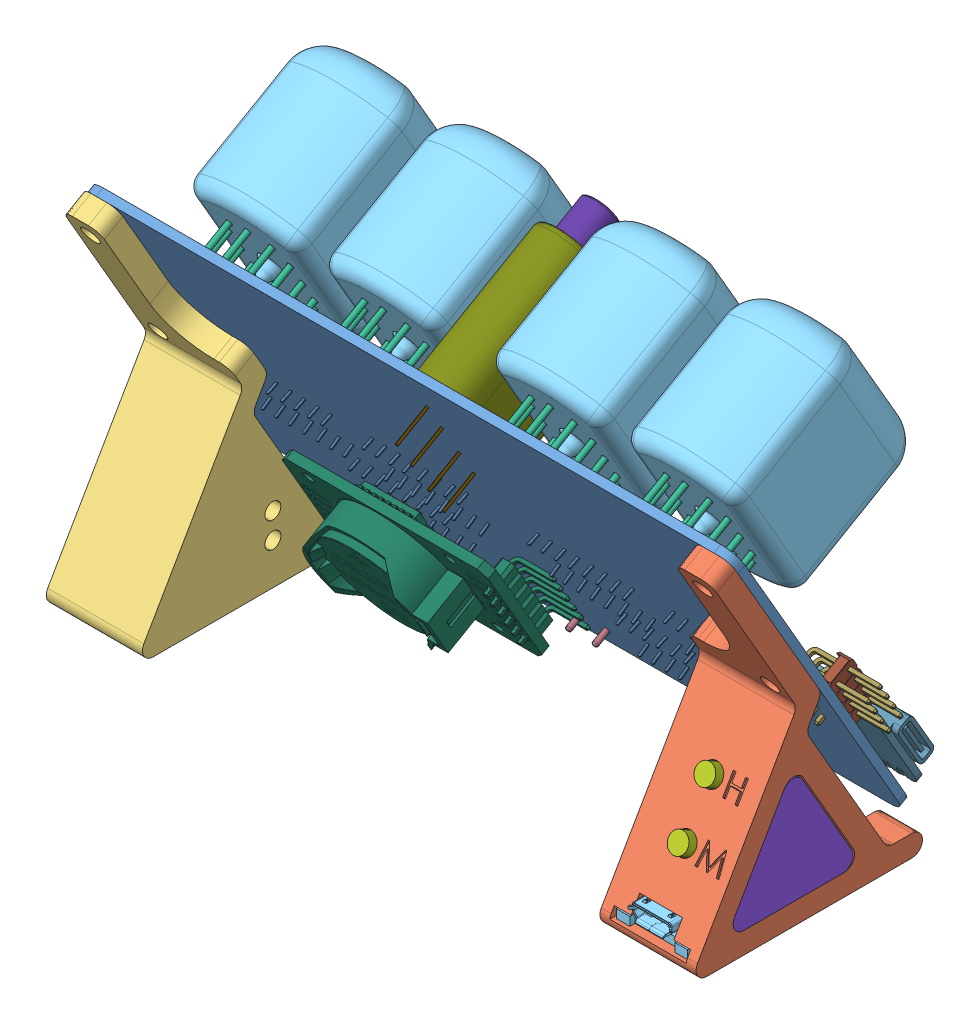
SolidWorks assembly assembly, configuration Défaut. Lengths in mm.
Overall size (130.66 87.93 77.4).
302 component instances, 62 part files, 31 mates.
Components (placement in the parent):
- nixie-display-1: nixie-display [Défaut] at (0 36.4164 17.774) x (-1 0 0) z (0 -0.866025 -0.5) size (127.16 50.53 67.27)
  - pcb-1: pcb [Défaut] at origin size (121.6 1.5 65.9)
  - IN-12A.stp-1: IN-12A.stp [Défaut] at (-40.9487 32.5 -15.5981) x (0 1 0) z (1 0 0) size (35 31 21)
    - 2.stp-1: 2.stp [Défaut] at origin size (2.7 24.17 15.83)
    - 3.stp-1: 3.stp [Défaut] at (-12.2 0 0) x (0 0 -1) z (-1 0 0) size (2 1.5 18.5)
    - 4.stp-1: 4.stp [Défaut] at (-12.2 0 0) x (0 0 1) z (-1 0 0) size (2 1.5 18.5)
    - 5.stp-1: 5.stp [Défaut] at (-12 0 0) x (0 0 -1) z (1 0 0) size (2.1 2.1 1)
    - 5.stp-2: 5.stp [Défaut] at (-10.8 0 0) x (0 0 -1) z (1 0 0) size (2.1 2.1 1)
    - 5.stp-3: 5.stp [Défaut] at (-9.6 0 0) x (0 0 -1) z (1 0 0) size (2.1 2.1 1)
    - 5.stp-4: 5.stp [Défaut] at (-8.4 0 0) x (0 0 -1) z (1 0 0) size (2.1 2.1 1)
    - 5.stp-5: 5.stp [Défaut] at (-7.2 0 0) x (0 0 -1) z (1 0 0) size (2.1 2.1 1)
    - 5.stp-6: 5.stp [Défaut] at (-6 0 0) x (0 0 -1) z (1 0 0) size (2.1 2.1 1)
    - 5.stp-7: 5.stp [Défaut] at (-4.8 0 0) x (0 0 -1) z (1 0 0) size (2.1 2.1 1)
    - 5.stp-8: 5.stp [Défaut] at (-3.6 0 0) x (0 0 -1) z (1 0 0) size (2.1 2.1 1)
    - 5.stp-9: 5.stp [Défaut] at (-2.4 0 0) x (0 0 -1) z (1 0 0) size (2.1 2.1 1)
    - 5.stp-10: 5.stp [Défaut] at (-1.2 0 0) x (0 0 -1) z (1 0 0) size (2.1 2.1 1)
    - 6.stp-1: 6.stp [Défaut] at (-11 16.1596 7.8778) x (0 -0.787778 0.61596) z (-1 0 0) size (2.1 2.1 1)
    - 7.stp-1: 7.stp [Défaut] at (-9.8 16.1596 7.8778) x (0 -0.787778 0.61596) z (-1 0 0) size (2.1 2.1 1)
    - 8.stp-1: 8.stp [Défaut] at (-8.6 16.1596 7.8778) x (0 -0.787778 0.61596) z (-1 0 0) size (2.1 2.1 1)
    - 9.stp-1: 9.stp [Défaut] at (-7.4 16.1596 7.8778) x (0 -0.787778 0.61596) z (-1 0 0) size (2.1 2.1 1)
    - 10.stp-1: 10.stp [Défaut] at (-6.2 16.1596 7.8778) x (0 -0.787778 0.61596) z (-1 0 0) size (2.1 2.1 1)
    - 11.stp-1: 11.stp [Défaut] at (-5 16.1596 7.8778) x (0 -0.787778 0.61596) z (-1 0 0) size (2.1 2.1 1)
    - 12.stp-1: 12.stp [Défaut] at (-3.8 16.1596 7.8778) x (0 -0.787778 0.61596) z (-1 0 0) size (2.1 2.1 1)
    - 13.stp-1: 13.stp [Défaut] at (-2.6 16.1596 7.8778) x (0 -0.787778 0.61596) z (-1 0 0) size (2.1 2.1 1)
    - 14.stp-1: 14.stp [Défaut] at (-1.4 16.1596 7.8778) x (0 -0.787778 0.61596) z (-1 0 0) size (2.1 2.1 1)
    - 15.stp-1: 15.stp [Défaut] at (-0.2 16.1596 7.8778) x (0 -0.787778 0.61596) z (-1 0 0) size (2.1 2.1 1)
    - 5.stp-11: 5.stp [Défaut] x (0 0 -1) z (1 0 0) size (2.1 2.1 1)
    - 5.stp-12: 5.stp [Défaut] at (-13.2 0 0) x (0 0 -1) z (1 0 0) size (2.1 2.1 1)
    - 16.stp-1: 16.stp [Défaut] at (1 16.1596 7.8778) x (0 -0.787778 0.61596) z (-1 0 0) size (2.1 2.1 1)
    - 17.stp-1: 17.stp [Défaut] at (-12.2 16.1596 7.8778) x (0 -0.787778 0.61596) z (-1 0 0) size (2.1 2.1 1)
    - 18.stp-1: 18.stp [Défaut] at (-13.2 0 0) x (0 0 -1) z (-1 0 0) size (15.83 24.17 12.28)
    - 19.stp-1: 19.stp [Défaut] x (1 0 0) z (0 1 0) size (1.51 1.46 20.68)
    - 20.stp-1: 20.stp [Défaut] at (1 0 0) size (4 22.27 2.42)
    - 21.stp-1: 21.stp [Défaut] at (-13.4 0 0) x (0 0 -1) z (-1 0 0) size (15.83 24.17 1)
    - 22.stp-1: 22.stp [Défaut] at (-14.4 0 0) x (0 0 -1) z (-1 0 0) size (15.83 27.29 2)
    - 23.stp-1: 23.stp [Défaut] x (0 0 -1) z (-1 0 0) size (21 31 33)
    - 24.stp-1: 24.stp [Défaut] x (0 0 -1) z (-1 0 0) size (1 1 15.5)
    - 24.stp-2: 24.stp [Défaut] at (0 -4.5 0) x (0 0 -1) z (-1 0 0) size (1 1 15.5)
    - 24.stp-3: 24.stp [Défaut] at (0 -8 -1.75) x (0 0 -1) z (-1 0 0) size (1 1 15.5)
    - 24.stp-4: 24.stp [Défaut] at (0 -9 -5.75) x (0 0 -1) z (-1 0 0) size (1 1 15.5)
    - 24.stp-5: 24.stp [Défaut] at (0 -8 -9.75) x (0 0 -1) z (-1 0 0) size (1 1 15.5)
    - 24.stp-6: 24.stp [Défaut] at (0 -4.5 -11.5) x (0 0 -1) z (-1 0 0) size (1 1 15.5)
    - 24.stp-7: 24.stp [Défaut] at (0 0 -11.5) x (0 0 -1) z (-1 0 0) size (1 1 15.5)
    - 24.stp-8: 24.stp [Défaut] at (0 4.5 -11.5) x (0 0 -1) z (-1 0 0) size (1 1 15.5)
    - 24.stp-9: 24.stp [Défaut] at (0 8 -9.75) x (0 0 -1) z (-1 0 0) size (1 1 15.5)
    - 24.stp-10: 24.stp [Défaut] at (0 9 -5.75) x (0 0 -1) z (-1 0 0) size (1 1 15.5)
    - 24.stp-11: 24.stp [Défaut] at (0 8 -1.75) x (0 0 -1) z (-1 0 0) size (1 1 15.5)
    - 24.stp-12: 24.stp [Défaut] at (0 4.5 0) x (0 0 -1) z (-1 0 0) size (1 1 15.5)
    - 25.stp-1: 25.stp [Défaut] at (-1.4 0 0) x (0 0 1) z (1 0 0) size (10.55 22 0.2)
    - 26.stp-1: 26.stp [Défaut] at (-2.6 0 0) x (0 0 1) z (1 0 0) size (11 22 0.2)
    - 27.stp-1: 27.stp [Défaut] at (-3.8 0 0) x (0 0 1) z (1 0 0) size (11 22 0.2)
    - 28.stp-1: 28.stp [Défaut] at (-5 0 0) x (0 0 1) z (1 0 0) size (10 22 0.2)
    - 29.stp-1: 29.stp [Défaut] at (-7.4 0 0) x (0 0 1) z (1 0 0) size (10 22 0.2)
    - 30.stp-1: 30.stp [Défaut] at (-9.6 0 0) x (0 0 -1) z (-1 0 0) size (10 22 0.2)
    - 31.stp-1: 31.stp [Défaut] at (-11 0 0) x (0 0 1) z (1 0 0) size (11 22 0.2)
    - 32.stp-1: 32.stp [Défaut] at (-12.2 0 0) x (0 0 1) z (1 0 0) size (2 22 0.2)
    - 33.stp-1: 33.stp [Défaut] at (-6 0 0) x (0 0 -1) z (-1 0 0) size (11 22 0.2)
    - 34.stp-1: 34.stp [Défaut] at (-8.6 0 0) x (0 0 1) z (1 0 0) size (10 22 0.2)
    - 1.stp-1: 1.stp [Défaut] at origin size (7.54 3.19 3.19)
    - 1-0.stp-1: 1-0.stp [Défaut] at origin size (11.99 9.11 6.32)
    - 1-1.stp-1: 1-1.stp [Défaut] at origin size (5.03 4.26 4.61)
    - 1-2.stp-1: 1-2.stp [Défaut] at origin size (8.17 8.42 6.65)
    - 1-3.stp-1: 1-3.stp [Défaut] at origin size (17.22 12.89 7.69)
    - 1-4.stp-1: 1-4.stp [Défaut] at origin size (13.11 12.81 7.39)
    - 1-5.stp-1: 1-5.stp [Défaut] at origin size (15.91 7.54 6.9)
    - 1-6.stp-1: 1-6.stp [Défaut] at origin size (10.39 4.47 4.23)
    - 1-7.stp-1: 1-7.stp [Défaut] at origin size (7.32 4.98 2.44)
    - 1-8.stp-1: 1-8.stp [Défaut] at origin size (10.29 4.36 5.63)
    - 1-9.stp-1: 1-9.stp [Défaut] at origin size (12.89 8.1 7.83)
  - IN-12A.stp-2: IN-12A.stp [Défaut] at (15.5408 32.5 -15.6508) x (0 1 0) z (1 0 0) size (35 31 21)
    - 2.stp-1: 2.stp [Défaut] at origin size (2.7 24.17 15.83)
    - 3.stp-1: 3.stp [Défaut] at (-12.2 0 0) x (0 0 -1) z (-1 0 0) size (2 1.5 18.5)
    - 4.stp-1: 4.stp [Défaut] at (-12.2 0 0) x (0 0 1) z (-1 0 0) size (2 1.5 18.5)
    - 5.stp-1: 5.stp [Défaut] at (-12 0 0) x (0 0 -1) z (1 0 0) size (2.1 2.1 1)
    - 5.stp-2: 5.stp [Défaut] at (-10.8 0 0) x (0 0 -1) z (1 0 0) size (2.1 2.1 1)
    - 5.stp-3: 5.stp [Défaut] at (-9.6 0 0) x (0 0 -1) z (1 0 0) size (2.1 2.1 1)
    - 5.stp-4: 5.stp [Défaut] at (-8.4 0 0) x (0 0 -1) z (1 0 0) size (2.1 2.1 1)
    - 5.stp-5: 5.stp [Défaut] at (-7.2 0 0) x (0 0 -1) z (1 0 0) size (2.1 2.1 1)
    - 5.stp-6: 5.stp [Défaut] at (-6 0 0) x (0 0 -1) z (1 0 0) size (2.1 2.1 1)
    - 5.stp-7: 5.stp [Défaut] at (-4.8 0 0) x (0 0 -1) z (1 0 0) size (2.1 2.1 1)
    - 5.stp-8: 5.stp [Défaut] at (-3.6 0 0) x (0 0 -1) z (1 0 0) size (2.1 2.1 1)
    - 5.stp-9: 5.stp [Défaut] at (-2.4 0 0) x (0 0 -1) z (1 0 0) size (2.1 2.1 1)
    - 5.stp-10: 5.stp [Défaut] at (-1.2 0 0) x (0 0 -1) z (1 0 0) size (2.1 2.1 1)
    - 6.stp-1: 6.stp [Défaut] at (-11 16.1596 7.8778) x (0 -0.787778 0.61596) z (-1 0 0) size (2.1 2.1 1)
    - 7.stp-1: 7.stp [Défaut] at (-9.8 16.1596 7.8778) x (0 -0.787778 0.61596) z (-1 0 0) size (2.1 2.1 1)
    - 8.stp-1: 8.stp [Défaut] at (-8.6 16.1596 7.8778) x (0 -0.787778 0.61596) z (-1 0 0) size (2.1 2.1 1)
    - 9.stp-1: 9.stp [Défaut] at (-7.4 16.1596 7.8778) x (0 -0.787778 0.61596) z (-1 0 0) size (2.1 2.1 1)
    - 10.stp-1: 10.stp [Défaut] at (-6.2 16.1596 7.8778) x (0 -0.787778 0.61596) z (-1 0 0) size (2.1 2.1 1)
    - 11.stp-1: 11.stp [Défaut] at (-5 16.1596 7.8778) x (0 -0.787778 0.61596) z (-1 0 0) size (2.1 2.1 1)
    - 12.stp-1: 12.stp [Défaut] at (-3.8 16.1596 7.8778) x (0 -0.787778 0.61596) z (-1 0 0) size (2.1 2.1 1)
    - 13.stp-1: 13.stp [Défaut] at (-2.6 16.1596 7.8778) x (0 -0.787778 0.61596) z (-1 0 0) size (2.1 2.1 1)
    - 14.stp-1: 14.stp [Défaut] at (-1.4 16.1596 7.8778) x (0 -0.787778 0.61596) z (-1 0 0) size (2.1 2.1 1)
    - 15.stp-1: 15.stp [Défaut] at (-0.2 16.1596 7.8778) x (0 -0.787778 0.61596) z (-1 0 0) size (2.1 2.1 1)
    - 5.stp-11: 5.stp [Défaut] x (0 0 -1) z (1 0 0) size (2.1 2.1 1)
    - 5.stp-12: 5.stp [Défaut] at (-13.2 0 0) x (0 0 -1) z (1 0 0) size (2.1 2.1 1)
    - 16.stp-1: 16.stp [Défaut] at (1 16.1596 7.8778) x (0 -0.787778 0.61596) z (-1 0 0) size (2.1 2.1 1)
    - 17.stp-1: 17.stp [Défaut] at (-12.2 16.1596 7.8778) x (0 -0.787778 0.61596) z (-1 0 0) size (2.1 2.1 1)
    - 18.stp-1: 18.stp [Défaut] at (-13.2 0 0) x (0 0 -1) z (-1 0 0) size (15.83 24.17 12.28)
    - 19.stp-1: 19.stp [Défaut] x (1 0 0) z (0 1 0) size (1.51 1.46 20.68)
    - 20.stp-1: 20.stp [Défaut] at (1 0 0) size (4 22.27 2.42)
    - 21.stp-1: 21.stp [Défaut] at (-13.4 0 0) x (0 0 -1) z (-1 0 0) size (15.83 24.17 1)
    - 22.stp-1: 22.stp [Défaut] at (-14.4 0 0) x (0 0 -1) z (-1 0 0) size (15.83 27.29 2)
    - 23.stp-1: 23.stp [Défaut] x (0 0 -1) z (-1 0 0) size (21 31 33)
    - 24.stp-1: 24.stp [Défaut] x (0 0 -1) z (-1 0 0) size (1 1 15.5)
    - 24.stp-2: 24.stp [Défaut] at (0 -4.5 0) x (0 0 -1) z (-1 0 0) size (1 1 15.5)
    - 24.stp-3: 24.stp [Défaut] at (0 -8 -1.75) x (0 0 -1) z (-1 0 0) size (1 1 15.5)
    - 24.stp-4: 24.stp [Défaut] at (0 -9 -5.75) x (0 0 -1) z (-1 0 0) size (1 1 15.5)
    - 24.stp-5: 24.stp [Défaut] at (0 -8 -9.75) x (0 0 -1) z (-1 0 0) size (1 1 15.5)
    - 24.stp-6: 24.stp [Défaut] at (0 -4.5 -11.5) x (0 0 -1) z (-1 0 0) size (1 1 15.5)
    - 24.stp-7: 24.stp [Défaut] at (0 0 -11.5) x (0 0 -1) z (-1 0 0) size (1 1 15.5)
    - 24.stp-8: 24.stp [Défaut] at (0 4.5 -11.5) x (0 0 -1) z (-1 0 0) size (1 1 15.5)
    - 24.stp-9: 24.stp [Défaut] at (0 8 -9.75) x (0 0 -1) z (-1 0 0) size (1 1 15.5)
    - 24.stp-10: 24.stp [Défaut] at (0 9 -5.75) x (0 0 -1) z (-1 0 0) size (1 1 15.5)
    - 24.stp-11: 24.stp [Défaut] at (0 8 -1.75) x (0 0 -1) z (-1 0 0) size (1 1 15.5)
    - 24.stp-12: 24.stp [Défaut] at (0 4.5 0) x (0 0 -1) z (-1 0 0) size (1 1 15.5)
    - 25.stp-1: 25.stp [Défaut] at (-1.4 0 0) x (0 0 1) z (1 0 0) size (10.55 22 0.2)
    - 26.stp-1: 26.stp [Défaut] at (-2.6 0 0) x (0 0 1) z (1 0 0) size (11 22 0.2)
    - 27.stp-1: 27.stp [Défaut] at (-3.8 0 0) x (0 0 1) z (1 0 0) size (11 22 0.2)
    - 28.stp-1: 28.stp [Défaut] at (-5 0 0) x (0 0 1) z (1 0 0) size (10 22 0.2)
    - 29.stp-1: 29.stp [Défaut] at (-7.4 0 0) x (0 0 1) z (1 0 0) size (10 22 0.2)
    - 30.stp-1: 30.stp [Défaut] at (-9.6 0 0) x (0 0 -1) z (-1 0 0) size (10 22 0.2)
    - 31.stp-1: 31.stp [Défaut] at (-11 0 0) x (0 0 1) z (1 0 0) size (11 22 0.2)
    - 32.stp-1: 32.stp [Défaut] at (-12.2 0 0) x (0 0 1) z (1 0 0) size (2 22 0.2)
    - 33.stp-1: 33.stp [Défaut] at (-6 0 0) x (0 0 -1) z (-1 0 0) size (11 22 0.2)
    - 34.stp-1: 34.stp [Défaut] at (-8.6 0 0) x (0 0 1) z (1 0 0) size (10 22 0.2)
    - 1.stp-1: 1.stp [Défaut] at origin size (7.54 3.19 3.19)
    - 1-0.stp-1: 1-0.stp [Défaut] at origin size (11.99 9.11 6.32)
    - 1-1.stp-1: 1-1.stp [Défaut] at origin size (5.03 4.26 4.61)
    - 1-2.stp-1: 1-2.stp [Défaut] at origin size (8.17 8.42 6.65)
    - 1-3.stp-1: 1-3.stp [Défaut] at origin size (17.22 12.89 7.69)
    - 1-4.stp-1: 1-4.stp [Défaut] at origin size (13.11 12.81 7.39)
    - 1-5.stp-1: 1-5.stp [Défaut] at origin size (15.91 7.54 6.9)
    - 1-6.stp-1: 1-6.stp [Défaut] at origin size (10.39 4.47 4.23)
    - 1-7.stp-1: 1-7.stp [Défaut] at origin size (7.32 4.98 2.44)
    - 1-8.stp-1: 1-8.stp [Défaut] at origin size (10.29 4.36 5.63)
    - 1-9.stp-1: 1-9.stp [Défaut] at origin size (12.89 8.1 7.83)
  - IN-12A.stp-3: IN-12A.stp [Défaut] at (-15.577 32.5 -15.4564) x (0 1 0) z (1 0 0) size (35 31 21)
    - 2.stp-1: 2.stp [Défaut] at origin size (2.7 24.17 15.83)
    - 3.stp-1: 3.stp [Défaut] at (-12.2 0 0) x (0 0 -1) z (-1 0 0) size (2 1.5 18.5)
    - 4.stp-1: 4.stp [Défaut] at (-12.2 0 0) x (0 0 1) z (-1 0 0) size (2 1.5 18.5)
    - 5.stp-1: 5.stp [Défaut] at (-12 0 0) x (0 0 -1) z (1 0 0) size (2.1 2.1 1)
    - 5.stp-2: 5.stp [Défaut] at (-10.8 0 0) x (0 0 -1) z (1 0 0) size (2.1 2.1 1)
    - 5.stp-3: 5.stp [Défaut] at (-9.6 0 0) x (0 0 -1) z (1 0 0) size (2.1 2.1 1)
    - 5.stp-4: 5.stp [Défaut] at (-8.4 0 0) x (0 0 -1) z (1 0 0) size (2.1 2.1 1)
    - 5.stp-5: 5.stp [Défaut] at (-7.2 0 0) x (0 0 -1) z (1 0 0) size (2.1 2.1 1)
    - 5.stp-6: 5.stp [Défaut] at (-6 0 0) x (0 0 -1) z (1 0 0) size (2.1 2.1 1)
    - 5.stp-7: 5.stp [Défaut] at (-4.8 0 0) x (0 0 -1) z (1 0 0) size (2.1 2.1 1)
    - 5.stp-8: 5.stp [Défaut] at (-3.6 0 0) x (0 0 -1) z (1 0 0) size (2.1 2.1 1)
    - 5.stp-9: 5.stp [Défaut] at (-2.4 0 0) x (0 0 -1) z (1 0 0) size (2.1 2.1 1)
    - 5.stp-10: 5.stp [Défaut] at (-1.2 0 0) x (0 0 -1) z (1 0 0) size (2.1 2.1 1)
    - 6.stp-1: 6.stp [Défaut] at (-11 16.1596 7.8778) x (0 -0.787778 0.61596) z (-1 0 0) size (2.1 2.1 1)
    - 7.stp-1: 7.stp [Défaut] at (-9.8 16.1596 7.8778) x (0 -0.787778 0.61596) z (-1 0 0) size (2.1 2.1 1)
    - 8.stp-1: 8.stp [Défaut] at (-8.6 16.1596 7.8778) x (0 -0.787778 0.61596) z (-1 0 0) size (2.1 2.1 1)
    - 9.stp-1: 9.stp [Défaut] at (-7.4 16.1596 7.8778) x (0 -0.787778 0.61596) z (-1 0 0) size (2.1 2.1 1)
    - 10.stp-1: 10.stp [Défaut] at (-6.2 16.1596 7.8778) x (0 -0.787778 0.61596) z (-1 0 0) size (2.1 2.1 1)
    - 11.stp-1: 11.stp [Défaut] at (-5 16.1596 7.8778) x (0 -0.787778 0.61596) z (-1 0 0) size (2.1 2.1 1)
    - 12.stp-1: 12.stp [Défaut] at (-3.8 16.1596 7.8778) x (0 -0.787778 0.61596) z (-1 0 0) size (2.1 2.1 1)
    - 13.stp-1: 13.stp [Défaut] at (-2.6 16.1596 7.8778) x (0 -0.787778 0.61596) z (-1 0 0) size (2.1 2.1 1)
    - 14.stp-1: 14.stp [Défaut] at (-1.4 16.1596 7.8778) x (0 -0.787778 0.61596) z (-1 0 0) size (2.1 2.1 1)
    - 15.stp-1: 15.stp [Défaut] at (-0.2 16.1596 7.8778) x (0 -0.787778 0.61596) z (-1 0 0) size (2.1 2.1 1)
    - 5.stp-11: 5.stp [Défaut] x (0 0 -1) z (1 0 0) size (2.1 2.1 1)
    - 5.stp-12: 5.stp [Défaut] at (-13.2 0 0) x (0 0 -1) z (1 0 0) size (2.1 2.1 1)
    - 16.stp-1: 16.stp [Défaut] at (1 16.1596 7.8778) x (0 -0.787778 0.61596) z (-1 0 0) size (2.1 2.1 1)
    - 17.stp-1: 17.stp [Défaut] at (-12.2 16.1596 7.8778) x (0 -0.787778 0.61596) z (-1 0 0) size (2.1 2.1 1)
    - 18.stp-1: 18.stp [Défaut] at (-13.2 0 0) x (0 0 -1) z (-1 0 0) size (15.83 24.17 12.28)
    - 19.stp-1: 19.stp [Défaut] x (1 0 0) z (0 1 0) size (1.51 1.46 20.68)
    - 20.stp-1: 20.stp [Défaut] at (1 0 0) size (4 22.27 2.42)
    - 21.stp-1: 21.stp [Défaut] at (-13.4 0 0) x (0 0 -1) z (-1 0 0) size (15.83 24.17 1)
    - 22.stp-1: 22.stp [Défaut] at (-14.4 0 0) x (0 0 -1) z (-1 0 0) size (15.83 27.29 2)
    - 23.stp-1: 23.stp [Défaut] x (0 0 -1) z (-1 0 0) size (21 31 33)
    - 24.stp-1: 24.stp [Défaut] x (0 0 -1) z (-1 0 0) size (1 1 15.5)
    - 24.stp-2: 24.stp [Défaut] at (0 -4.5 0) x (0 0 -1) z (-1 0 0) size (1 1 15.5)
    - 24.stp-3: 24.stp [Défaut] at (0 -8 -1.75) x (0 0 -1) z (-1 0 0) size (1 1 15.5)
    - 24.stp-4: 24.stp [Défaut] at (0 -9 -5.75) x (0 0 -1) z (-1 0 0) size (1 1 15.5)
    - 24.stp-5: 24.stp [Défaut] at (0 -8 -9.75) x (0 0 -1) z (-1 0 0) size (1 1 15.5)
    - 24.stp-6: 24.stp [Défaut] at (0 -4.5 -11.5) x (0 0 -1) z (-1 0 0) size (1 1 15.5)
    - 24.stp-7: 24.stp [Défaut] at (0 0 -11.5) x (0 0 -1) z (-1 0 0) size (1 1 15.5)
    - 24.stp-8: 24.stp [Défaut] at (0 4.5 -11.5) x (0 0 -1) z (-1 0 0) size (1 1 15.5)
    - 24.stp-9: 24.stp [Défaut] at (0 8 -9.75) x (0 0 -1) z (-1 0 0) size (1 1 15.5)
    - 24.stp-10: 24.stp [Défaut] at (0 9 -5.75) x (0 0 -1) z (-1 0 0) size (1 1 15.5)
    - 24.stp-11: 24.stp [Défaut] at (0 8 -1.75) x (0 0 -1) z (-1 0 0) size (1 1 15.5)
    - 24.stp-12: 24.stp [Défaut] at (0 4.5 0) x (0 0 -1) z (-1 0 0) size (1 1 15.5)
    - 25.stp-1: 25.stp [Défaut] at (-1.4 0 0) x (0 0 1) z (1 0 0) size (10.55 22 0.2)
    - 26.stp-1: 26.stp [Défaut] at (-2.6 0 0) x (0 0 1) z (1 0 0) size (11 22 0.2)
    - 27.stp-1: 27.stp [Défaut] at (-3.8 0 0) x (0 0 1) z (1 0 0) size (11 22 0.2)
    - 28.stp-1: 28.stp [Défaut] at (-5 0 0) x (0 0 1) z (1 0 0) size (10 22 0.2)
    - 29.stp-1: 29.stp [Défaut] at (-7.4 0 0) x (0 0 1) z (1 0 0) size (10 22 0.2)
    - 30.stp-1: 30.stp [Défaut] at (-9.6 0 0) x (0 0 -1) z (-1 0 0) size (10 22 0.2)
    - 31.stp-1: 31.stp [Défaut] at (-11 0 0) x (0 0 1) z (1 0 0) size (11 22 0.2)
    - 32.stp-1: 32.stp [Défaut] at (-12.2 0 0) x (0 0 1) z (1 0 0) size (2 22 0.2)
    - 33.stp-1: 33.stp [Défaut] at (-6 0 0) x (0 0 -1) z (-1 0 0) size (11 22 0.2)
    - 34.stp-1: 34.stp [Défaut] at (-8.6 0 0) x (0 0 1) z (1 0 0) size (10 22 0.2)
    - 1.stp-1: 1.stp [Défaut] at origin size (7.54 3.19 3.19)
    - 1-0.stp-1: 1-0.stp [Défaut] at origin size (11.99 9.11 6.32)
    - 1-1.stp-1: 1-1.stp [Défaut] at origin size (5.03 4.26 4.61)
    - 1-2.stp-1: 1-2.stp [Défaut] at origin size (8.17 8.42 6.65)
    - 1-3.stp-1: 1-3.stp [Défaut] at origin size (17.22 12.89 7.69)
    - 1-4.stp-1: 1-4.stp [Défaut] at origin size (13.11 12.81 7.39)
    - 1-5.stp-1: 1-5.stp [Défaut] at origin size (15.91 7.54 6.9)
    - 1-6.stp-1: 1-6.stp [Défaut] at origin size (10.39 4.47 4.23)
    - 1-7.stp-1: 1-7.stp [Défaut] at origin size (7.32 4.98 2.44)
    - 1-8.stp-1: 1-8.stp [Défaut] at origin size (10.29 4.36 5.63)
    - 1-9.stp-1: 1-9.stp [Défaut] at origin size (12.89 8.1 7.83)
  - IN-12A.stp-4: IN-12A.stp [Défaut] at (40.934 32.5 -15.666) x (0 1 0) z (1 0 0) size (35 31 21)
    - 2.stp-1: 2.stp [Défaut] at origin size (2.7 24.17 15.83)
    - 3.stp-1: 3.stp [Défaut] at (-12.2 0 0) x (0 0 -1) z (-1 0 0) size (2 1.5 18.5)
    - 4.stp-1: 4.stp [Défaut] at (-12.2 0 0) x (0 0 1) z (-1 0 0) size (2 1.5 18.5)
    - 5.stp-1: 5.stp [Défaut] at (-12 0 0) x (0 0 -1) z (1 0 0) size (2.1 2.1 1)
    - 5.stp-2: 5.stp [Défaut] at (-10.8 0 0) x (0 0 -1) z (1 0 0) size (2.1 2.1 1)
    - 5.stp-3: 5.stp [Défaut] at (-9.6 0 0) x (0 0 -1) z (1 0 0) size (2.1 2.1 1)
    - 5.stp-4: 5.stp [Défaut] at (-8.4 0 0) x (0 0 -1) z (1 0 0) size (2.1 2.1 1)
    - 5.stp-5: 5.stp [Défaut] at (-7.2 0 0) x (0 0 -1) z (1 0 0) size (2.1 2.1 1)
    - 5.stp-6: 5.stp [Défaut] at (-6 0 0) x (0 0 -1) z (1 0 0) size (2.1 2.1 1)
    - 5.stp-7: 5.stp [Défaut] at (-4.8 0 0) x (0 0 -1) z (1 0 0) size (2.1 2.1 1)
    - 5.stp-8: 5.stp [Défaut] at (-3.6 0 0) x (0 0 -1) z (1 0 0) size (2.1 2.1 1)
    - 5.stp-9: 5.stp [Défaut] at (-2.4 0 0) x (0 0 -1) z (1 0 0) size (2.1 2.1 1)
    - 5.stp-10: 5.stp [Défaut] at (-1.2 0 0) x (0 0 -1) z (1 0 0) size (2.1 2.1 1)
    - 6.stp-1: 6.stp [Défaut] at (-11 16.1596 7.8778) x (0 -0.787778 0.61596) z (-1 0 0) size (2.1 2.1 1)
    - 7.stp-1: 7.stp [Défaut] at (-9.8 16.1596 7.8778) x (0 -0.787778 0.61596) z (-1 0 0) size (2.1 2.1 1)
    - 8.stp-1: 8.stp [Défaut] at (-8.6 16.1596 7.8778) x (0 -0.787778 0.61596) z (-1 0 0) size (2.1 2.1 1)
    - 9.stp-1: 9.stp [Défaut] at (-7.4 16.1596 7.8778) x (0 -0.787778 0.61596) z (-1 0 0) size (2.1 2.1 1)
    - 10.stp-1: 10.stp [Défaut] at (-6.2 16.1596 7.8778) x (0 -0.787778 0.61596) z (-1 0 0) size (2.1 2.1 1)
    - 11.stp-1: 11.stp [Défaut] at (-5 16.1596 7.8778) x (0 -0.787778 0.61596) z (-1 0 0) size (2.1 2.1 1)
    - 12.stp-1: 12.stp [Défaut] at (-3.8 16.1596 7.8778) x (0 -0.787778 0.61596) z (-1 0 0) size (2.1 2.1 1)
    - 13.stp-1: 13.stp [Défaut] at (-2.6 16.1596 7.8778) x (0 -0.787778 0.61596) z (-1 0 0) size (2.1 2.1 1)
    - 14.stp-1: 14.stp [Défaut] at (-1.4 16.1596 7.8778) x (0 -0.787778 0.61596) z (-1 0 0) size (2.1 2.1 1)
    - 15.stp-1: 15.stp [Défaut] at (-0.2 16.1596 7.8778) x (0 -0.787778 0.61596) z (-1 0 0) size (2.1 2.1 1)
    - 5.stp-11: 5.stp [Défaut] x (0 0 -1) z (1 0 0) size (2.1 2.1 1)
    - 5.stp-12: 5.stp [Défaut] at (-13.2 0 0) x (0 0 -1) z (1 0 0) size (2.1 2.1 1)
    - 16.stp-1: 16.stp [Défaut] at (1 16.1596 7.8778) x (0 -0.787778 0.61596) z (-1 0 0) size (2.1 2.1 1)
    - 17.stp-1: 17.stp [Défaut] at (-12.2 16.1596 7.8778) x (0 -0.787778 0.61596) z (-1 0 0) size (2.1 2.1 1)
    - 18.stp-1: 18.stp [Défaut] at (-13.2 0 0) x (0 0 -1) z (-1 0 0) size (15.83 24.17 12.28)
    - 19.stp-1: 19.stp [Défaut] x (1 0 0) z (0 1 0) size (1.51 1.46 20.68)
    - 20.stp-1: 20.stp [Défaut] at (1 0 0) size (4 22.27 2.42)
    - 21.stp-1: 21.stp [Défaut] at (-13.4 0 0) x (0 0 -1) z (-1 0 0) size (15.83 24.17 1)
    - 22.stp-1: 22.stp [Défaut] at (-14.4 0 0) x (0 0 -1) z (-1 0 0) size (15.83 27.29 2)
    - 23.stp-1: 23.stp [Défaut] x (0 0 -1) z (-1 0 0) size (21 31 33)
    - 24.stp-1: 24.stp [Défaut] x (0 0 -1) z (-1 0 0) size (1 1 15.5)
    - 24.stp-2: 24.stp [Défaut] at (0 -4.5 0) x (0 0 -1) z (-1 0 0) size (1 1 15.5)
    - 24.stp-3: 24.stp [Défaut] at (0 -8 -1.75) x (0 0 -1) z (-1 0 0) size (1 1 15.5)
    - 24.stp-4: 24.stp [Défaut] at (0 -9 -5.75) x (0 0 -1) z (-1 0 0) size (1 1 15.5)
    - 24.stp-5: 24.stp [Défaut] at (0 -8 -9.75) x (0 0 -1) z (-1 0 0) size (1 1 15.5)
    - 24.stp-6: 24.stp [Défaut] at (0 -4.5 -11.5) x (0 0 -1) z (-1 0 0) size (1 1 15.5)
    - 24.stp-7: 24.stp [Défaut] at (0 0 -11.5) x (0 0 -1) z (-1 0 0) size (1 1 15.5)
    - 24.stp-8: 24.stp [Défaut] at (0 4.5 -11.5) x (0 0 -1) z (-1 0 0) size (1 1 15.5)
    - 24.stp-9: 24.stp [Défaut] at (0 8 -9.75) x (0 0 -1) z (-1 0 0) size (1 1 15.5)
    - 24.stp-10: 24.stp [Défaut] at (0 9 -5.75) x (0 0 -1) z (-1 0 0) size (1 1 15.5)
    - 24.stp-11: 24.stp [Défaut] at (0 8 -1.75) x (0 0 -1) z (-1 0 0) size (1 1 15.5)
    - 24.stp-12: 24.stp [Défaut] at (0 4.5 0) x (0 0 -1) z (-1 0 0) size (1 1 15.5)
    - 25.stp-1: 25.stp [Défaut] at (-1.4 0 0) x (0 0 1) z (1 0 0) size (10.55 22 0.2)
    - 26.stp-1: 26.stp [Défaut] at (-2.6 0 0) x (0 0 1) z (1 0 0) size (11 22 0.2)
    - 27.stp-1: 27.stp [Défaut] at (-3.8 0 0) x (0 0 1) z (1 0 0) size (11 22 0.2)
    - 28.stp-1: 28.stp [Défaut] at (-5 0 0) x (0 0 1) z (1 0 0) size (10 22 0.2)
    - 29.stp-1: 29.stp [Défaut] at (-7.4 0 0) x (0 0 1) z (1 0 0) size (10 22 0.2)
    - 30.stp-1: 30.stp [Défaut] at (-9.6 0 0) x (0 0 -1) z (-1 0 0) size (10 22 0.2)
    - 31.stp-1: 31.stp [Défaut] at (-11 0 0) x (0 0 1) z (1 0 0) size (11 22 0.2)
    - 32.stp-1: 32.stp [Défaut] at (-12.2 0 0) x (0 0 1) z (1 0 0) size (2 22 0.2)
    - 33.stp-1: 33.stp [Défaut] at (-6 0 0) x (0 0 -1) z (-1 0 0) size (11 22 0.2)
    - 34.stp-1: 34.stp [Défaut] at (-8.6 0 0) x (0 0 1) z (1 0 0) size (10 22 0.2)
    - 1.stp-1: 1.stp [Défaut] at origin size (7.54 3.19 3.19)
    - 1-0.stp-1: 1-0.stp [Défaut] at origin size (11.99 9.11 6.32)
    - 1-1.stp-1: 1-1.stp [Défaut] at origin size (5.03 4.26 4.61)
    - 1-2.stp-1: 1-2.stp [Défaut] at origin size (8.17 8.42 6.65)
    - 1-3.stp-1: 1-3.stp [Défaut] at origin size (17.22 12.89 7.69)
    - 1-4.stp-1: 1-4.stp [Défaut] at origin size (13.11 12.81 7.39)
    - 1-5.stp-1: 1-5.stp [Défaut] at origin size (15.91 7.54 6.9)
    - 1-6.stp-1: 1-6.stp [Défaut] at origin size (10.39 4.47 4.23)
    - 1-7.stp-1: 1-7.stp [Défaut] at origin size (7.32 4.98 2.44)
    - 1-8.stp-1: 1-8.stp [Défaut] at origin size (10.29 4.36 5.63)
    - 1-9.stp-1: 1-9.stp [Défaut] at origin size (12.89 8.1 7.83)
  - DIP18N.step-1: DIP18N.step [Défaut] at (-50.7835 3.7087 35.4382) x (0 0 1) z (-1 0 0) size (8.53 6.85 19.5)
  - DIP18N.step-2: DIP18N.step [Défaut] at (31.1067 3.7087 35.4997) x (0 0 1) z (-1 0 0) size (8.53 6.85 19.5)
  - DIP18N.step-3: DIP18N.step [Défaut] at (5.6608 3.7087 35.5611) x (0 0 1) z (-1 0 0) size (8.53 6.85 19.5)
  - DIP18N.step-4: DIP18N.step [Défaut] at (-25.3559 3.7087 35.5399) x (0 0 1) z (-1 0 0) size (8.53 6.85 19.5)
  - DS1022-2x4RF11.stp-1: DS1022-2x4RF11.stp [Défaut] at (-56.1796 1.5 3.5604) x (0 0 1) z (0 1 0) size (10.16 13.04 8)
    - eBom-prt0.stp-1: eBom-prt0.stp [Défaut] at origin size (10.16 2.5 5)
    - eBom-prt1.stp-1: eBom-prt1.stp [Défaut] at origin size (0.64 13.04 7.09)
    - eBom-prt1.stp-2: eBom-prt1.stp [Défaut] at (2.54 0 0) size (0.64 13.04 7.09)
    - eBom-prt1.stp-3: eBom-prt1.stp [Défaut] at (5.08 0 0) size (0.64 13.04 7.09)
    - eBom-prt1.stp-4: eBom-prt1.stp [Défaut] at (7.62 0 0) size (0.64 13.04 7.09)
  - DIP18N.step-5: DIP18N.step [Défaut] at (-15.751 3.7087 -7.8923) x (0.008727 0 -0.999962) z (0.999962 0 0.008727) size (8.53 6.85 19.5)
  - DIP18N.step-6: DIP18N.step [Défaut] at (34.3108 3.7087 -7.8662) x (0.008727 0 -0.999962) z (0.999962 0 0.008727) size (8.53 6.85 19.5)
  - Screw Terminal Block 5mm-2: Screw Terminal Block 5mm [Valor predeterminado] at (0.4217 1.5 23.933) x (-0.999962 0 -0.008727) z (0.008727 0 -0.999962) size (10.6 16.9 9)
  - Seeeduino Xiao.step-1: Seeeduino Xiao.step [Défaut] at (-88.5187 11.44 25.9289) x (-0.008727 0 0.999962) z (-0.999962 0 -0.008727) size (17.8 4.27 22.5)
  - DS3231 RTC.step-1: DS3231 RTC.step [Défaut] at (21.2627 -4.62 22.922) x (1 0 0) z (0 1 0) size (44.75 22.8 13.53)
  - indics-1: indics [Défaut] at (0 1.5 -21.8057) size (10.8 43.17 23.8)
    - indic-holder-1: indic-holder [Défaut] at (0 0 6) size (10.8 28.02 23.8)
    - INS1.STEP-1: INS1.STEP [Défaut] at (0 17 0) x (0 0 1) z (-1 0 0) size (7.01 43.17 6.51)
      - INS1-Glask_rper_01.STEP-1: INS1-Glask_rper_01.STEP [Défaut] at origin size (7.01 28.6 6.51)
      - INS1_Inlay_01.STEP-1: INS1_Inlay_01.STEP [Défaut] at (0 5.1 0) size (6 41.77 5.25)
    - INS1.STEP-2: INS1.STEP [Défaut] at (0 17 12) x (0 0 1) z (-1 0 0) size (7.01 43.17 6.51)
      - INS1-Glask_rper_01.STEP-1: INS1-Glask_rper_01.STEP [Défaut] at origin size (7.01 28.6 6.51)
      - INS1_Inlay_01.STEP-1: INS1_Inlay_01.STEP [Défaut] at (0 5.1 0) size (6 41.77 5.25)
- hv-cover-1: hv-cover [Défaut] at (-59.2 20.5901 2.2859) x (-1 0 0) z (0 0.5 -0.866025) size (20.6 23 8)
- leg-left-1: leg-left [Défaut] at (42.8 0 -3.251) size (18 64.95 42.38)
- leg-right-1: leg-right [Défaut] at (-60.8 0 -3.251) size (18 64.95 42.38)
- plate-right-1: plate-right [Défaut] at (-56.7 4.2252 22.2905) x (0 0 1) z (-1 0 0) size (21.97 19.56 3.5)
- Micro-USB_breakout.step-1: Micro-USB_breakout.step [Défaut] at (58.45 3.8 39.8564) x (0 0 -1) z (0 1 0) size (16.21 13.3 4.6)
- Push Button WHITE-1: Push Button WHITE [Default] at (-55.4 10.1 22.2905) x (0 0 1) z (0 -1 0) size (13 15.4 13)
- 6x6 mm-1: 6x6 mm [Défaut] at (51.8 13.5942 31.9004) x (1 0 0) z (0 -0.866025 0.5) size (8.15 10.4 6.02)
- 6x6 mm-2: 6x6 mm [Défaut] at (51.8 22.2545 26.9004) x (1 0 0) z (0 -0.866025 0.5) size (8.15 10.4 6.02)
- plate-left-1: plate-left [Défaut] at (60.8 14.9985 28.7802) x (0 0.866025 -0.5) z (-1 0 0) size (22.47 20 3.5)
Mates (geometry in assembly coordinates):
- Coïncidente11: coincident anti-aligned: plane of nixie-display-1 through (0 36.4164 17.774) normal (-1 0 0)
- Coïncidente14: coincident: line of nixie-display-1/pcb-1 through (115.6 57.8 8.6308) axis (0 -1 0)
- Coïncidente15: coincident anti-aligned: plane of nixie-display-1/pcb-1 through (0 36.4164 17.774) normal (0 -0.5 0.866025); plane of leg-io-1 through (60.8 64.9519 34.249) normal (0 0.5 -0.866025)
- Coïncidente17: coincident anti-aligned: plane of leg-io-1 through (60.8 0 42.0584) normal (0 -1 0)
- Coïncidente18: coincident anti-aligned: line of nixie-display-1/pcb-1 through (-57.8 64.9519 34.249) axis (1 0 0); line of leg-io-1 through (58.8 64.9519 34.249) axis (-1 0 0)
- Coïncidente19: coincident anti-aligned: plane of leg-io-1 through (42.8 2.2 -3.251) normal (0 1 0); plane of Micro-USB_breakout.step-1 through (51.8039 2.2 32.1496) normal (0 -1 0)
- Coïncidente20: coincident anti-aligned: plane of leg-io-1 through (44.65 2.2 24.249) normal (0 0 1); plane of Micro-USB_breakout.step-1 through (58.45 3.8 24.249) normal (0 0 -1)
- Largeur2: width anti-aligned: plane of leg-io-1 through (44.65 2.2 42.0584) normal (1 0 0); plane of leg-io-1 through (58.95 2.2 42.0584) normal (-1 0 0); plane of Micro-USB_breakout.step-1 through (45.15 3.8 24.249) normal (-1 0 0); plane of Micro-USB_breakout.step-1 through (58.45 3.8 39.8564) normal (1 0 0)
- Coaxiale1: concentric anti-aligned: cylinder of leg-io-1 through (51.8 3.6343 -5.3508) axis (0 0.5 0.866025) radius 2; cylinder of 6x6 mm-2 through (51.8 22.2545 26.9004) axis (0 -0.5 -0.866025) radius 1.82
- Coïncidente23: coincident anti-aligned: plane of leg-io-1 through (42.8 18.6195 28.999) normal (0 -0.5 -0.866025); plane of 6x6 mm-2 through (51.8 22.2545 26.9004) normal (0 0.5 0.866025)
- Parallèle2: parallel aligned: plane of leg-io-1 through (60.8 0 -3.251) normal (1 0 0); plane of 6x6 mm-2 through (54.8 24.8526 25.4004) normal (1 0 0)
- Coïncidente25: coincident anti-aligned: plane of leg-io-1 through (42.8 18.6195 28.999) normal (0 -0.5 -0.866025); plane of 6x6 mm-1 through (51.8 13.5942 31.9004) normal (0 0.5 0.866025)
- Coaxiale2: concentric anti-aligned: cylinder of leg-io-1 through (51.8 -5.026 -0.3508) axis (0 0.5 0.866025) radius 2; cylinder of 6x6 mm-1 through (51.8 13.5942 31.9004) axis (0 -0.5 -0.866025) radius 1.82
- Coïncidente26: coincident aligned: plane of 6x6 mm-1 through (54.8 16.1923 30.4004) normal (1 0 0); plane of 6x6 mm-2 through (54.8 24.8526 25.4004) normal (1 0 0)
- Coïncidente27: coincident anti-aligned: plane of nixie-display-1/pcb-1 through (0 36.4164 17.774) normal (0 -0.5 0.866025); plane of leg-button-1 through (-42.8 64.9519 34.249) normal (0 0.5 -0.866025)
- Coïncidente28: coincident aligned: plane of leg-io-1 through (60.8 0 42.0584) normal (0 -1 0); plane of leg-button-1 through (-42.8 0 42.0584) normal (0 -1 0)
- Coïncidente29: coincident aligned: plane of nixie-display-1/pcb-1 through (-60.8 65.7019 32.95) normal (-1 0 0); plane of leg-button-1 through (-60.8 0 -3.251) normal (-1 0 0)
- Coïncidente30: coincident aligned: plane of nixie-display-1/pcb-1 through (60.8 65.7019 32.95) normal (1 0 0); plane of leg-io-1 through (60.8 0 -3.251) normal (1 0 0)
- Parallèle3: parallel aligned: plane of Push Button WHITE-1 through (-64.3 4.9 22.2905) normal (-1 0 0); plane of leg-button-1 through (-60.8 0 -3.251) normal (-1 0 0)
- Largeur5: width aligned: plane of Push Button WHITE-1 through (-52.4 4.13 16.3205) normal (0 -1 0); plane of Push Button WHITE-1 through (-52.4 16.07 16.3205) normal (0 1 0); plane of leg-button-1 through (-52.4 16.2 17.1905) normal (0 -1 0); plane of leg-button-1 through (-52.4 4 17.1905) normal (0 1 0)
- Coïncidente35: coincident anti-aligned: plane of Push Button WHITE-1 through (-52.4 10.1 22.2905) normal (1 0 0); plane of leg-button-1 through (-52.4 12.5 28.3905) normal (-1 0 0)
- Largeur6: width anti-aligned: plane of Push Button WHITE-1 through (-52.4 16.07 16.3205) normal (0 0 -1); plane of Push Button WHITE-1 through (-52.4 16.07 28.2605) normal (0 0 1); plane of leg-button-1 through (-52.4 6.8 16.1905) normal (0 0 1); plane of leg-button-1 through (-52.4 6.8 28.3905) normal (0 0 -1)
- Largeur3: width anti-aligned: plane of button-plate-1 through (-65.8569 12.1 24.2905) normal (0 -1 0); plane of button-plate-1 through (-65.8569 8.1 24.2905) normal (0 1 0); plane of Push Button WHITE-1 through (-59.6 12.025 20.5655) normal (0 1 0); plane of Push Button WHITE-1 through (-59.6 8.175 20.5655) normal (0 -1 0)
- Largeur4: width anti-aligned: plane of button-plate-1 through (-65.8569 12.1 20.2905) normal (0 0 1); plane of button-plate-1 through (-65.8569 12.1 24.2905) normal (0 0 -1); plane of Push Button WHITE-1 through (-59.6 11.825 20.3655) normal (0 0 -1); plane of Push Button WHITE-1 through (-59.6 11.825 24.2155) normal (0 0 1)
- Coïncidente40: coincident anti-aligned: plane of Push Button WHITE-1 through (-59.6 11.825 20.5655) normal (-1 0 0); plane of button-plate-1 through (-59.6 4.2252 22.2905) normal (1 0 0)
- Coïncidente41: coincident anti-aligned: plane of nixie-display-1/pcb-1 through (0 37.1664 16.475) normal (0 0.5 -0.866025); plane of cover-1 through (-60.8 28.5494 11.5) normal (0 -0.5 0.866025)
- Coïncidente42: coincident aligned: plane of nixie-display-1/pcb-1 through (-60.8 65.7019 32.95) normal (-1 0 0); plane of cover-1 through (-60.8 20.5901 2.2859) normal (-1 0 0)
- Coïncidente43: coincident aligned: plane of nixie-display-1/pcb-1 through (60.8 8.6308 0) normal (0 -0.866025 -0.5); plane of cover-1 through (-60.8 12.6308 -6.9282) normal (0 -0.866025 -0.5)
- Coïncidente44: coincident aligned: plane of leg-left-1 through (60.8 0 -3.251) normal (1 0 0); plane of left-plate-1 through (60.8 14.9985 28.7802) normal (1 0 0)
- Coïncidente45: coincident anti-aligned: plane of leg-left-1 through (60.8 4 35.1302) normal (0 1 0); plane of left-plate-1 through (57.3 4 9.7302) normal (0 -1 0)
- Coïncidente46: coincident anti-aligned: plane of leg-left-1 through (60.8 26.2391 22.2905) normal (0 -0.5 -0.866025); plane of left-plate-1 through (57.3 4 35.1302) normal (0 0.5 0.866025)
